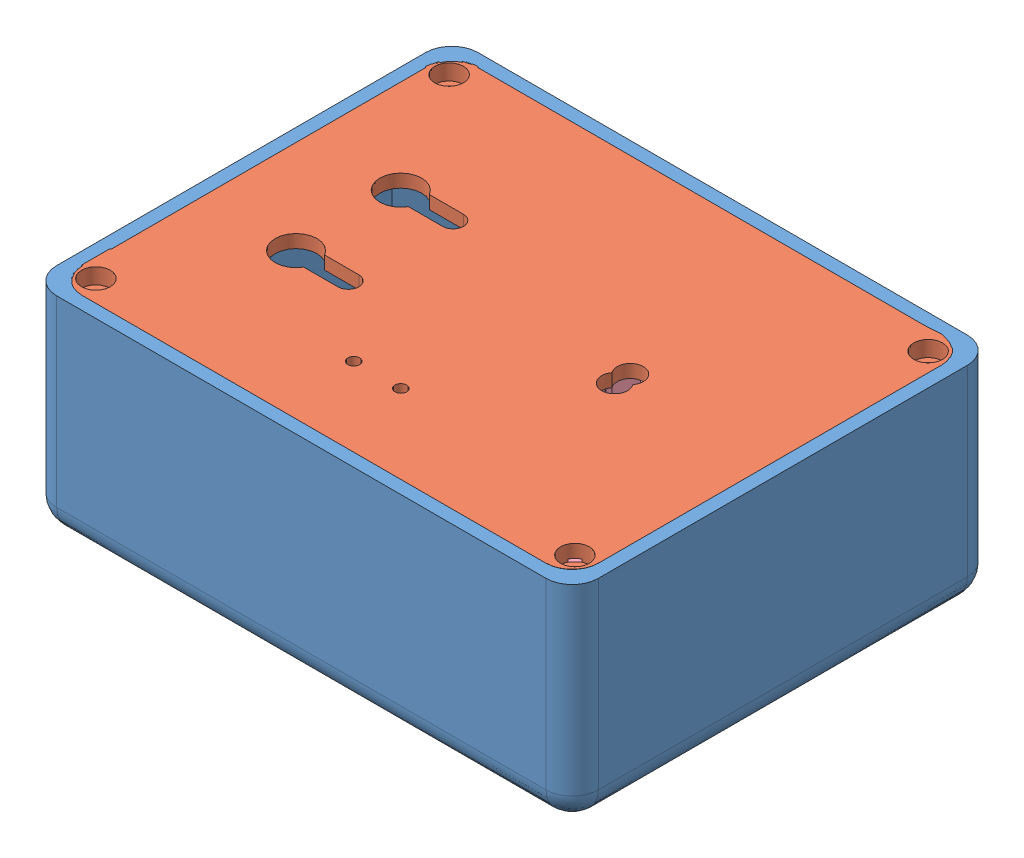
SolidWorks assembly Final_Assembly, configuration Default. Lengths in mm.
Overall size (103.47 42.5 80.48).
4 component instances, 4 part files, 8 mates.
Components (placement in the parent):
- Enclosure_Main-1: Enclosure_Main [Default] at (-4.226 28.3562 82.9036) x (1 0 0) z (0 -1 0) size (103.47 80.48 40)
- Cover-1: Cover [Default] at (-4.326 60.8562 82.8036) x (-1 0 0) z (0 1 0) size (98.67 75.69 25.5)
- OLED_Cover-1: OLED_Cover [Default] at (-4.303 25.8562 82.9038) x (1 0 0) z (0 -1 0) size (30 39.49 7.5)
- PCB-1: PCB [Default] at (89.246 36.2677 118.1461) x (0 0 -1) z (0 1 0) size (70.48 93.47 35.55)
Mates (geometry in assembly coordinates):
- Concentric1: concentric anti-aligned: circle of Enclosure_Main-1; circle of PCB-1
- Concentric2: concentric aligned: circle of Enclosure_Main-1; circle of PCB-1
- Coincident7: coincident anti-aligned: plane of Enclosure_Main-1 through (-4.226 25.8562 82.9036) normal (0 -1 0); plane of OLED_Cover-1 through (-4.303 25.8562 82.9038) normal (0 1 0)
- Width1: width anti-aligned: plane of OLED_Cover-1 through (-4.303 30.8562 102.6462) normal (0 0 1); plane of OLED_Cover-1 through (-4.303 30.8562 63.161) normal (0 0 -1); plane of Enclosure_Main-1 through (0.874 25.8562 102.7464) normal (0 0 -1); plane of Enclosure_Main-1 through (0.874 25.8562 63.0609) normal (0 0 1)
- Coincident12: coincident anti-aligned: plane of Enclosure_Main-1 through (-1.726 60.8562 115.6461) normal (0 1 0); plane of Cover-1 through (15.8277 60.8562 50.0611) normal (0 -1 0)
- Coincident13: coincident anti-aligned: plane of Enclosure_Main-1 through (80.2815 65.8562 120.6461) normal (0 0 -1); plane of Cover-1 through (15.8277 190.2121 120.6461) normal (0 0 1)
- Coincident14: coincident anti-aligned: plane of Enclosure_Main-1 through (91.746 65.8562 56.6256) normal (-1 0 0); plane of Cover-1 through (109.3997 190.2121 115.5461) normal (1 0 0)
- Distance1: distance = 5 mm anti-aligned: plane of OLED_Cover-1 through (-4.303 30.8562 82.9038) normal (0 1 0); plane of PCB-1 through (42.51 35.8562 82.9036) normal (0 -1 0)
